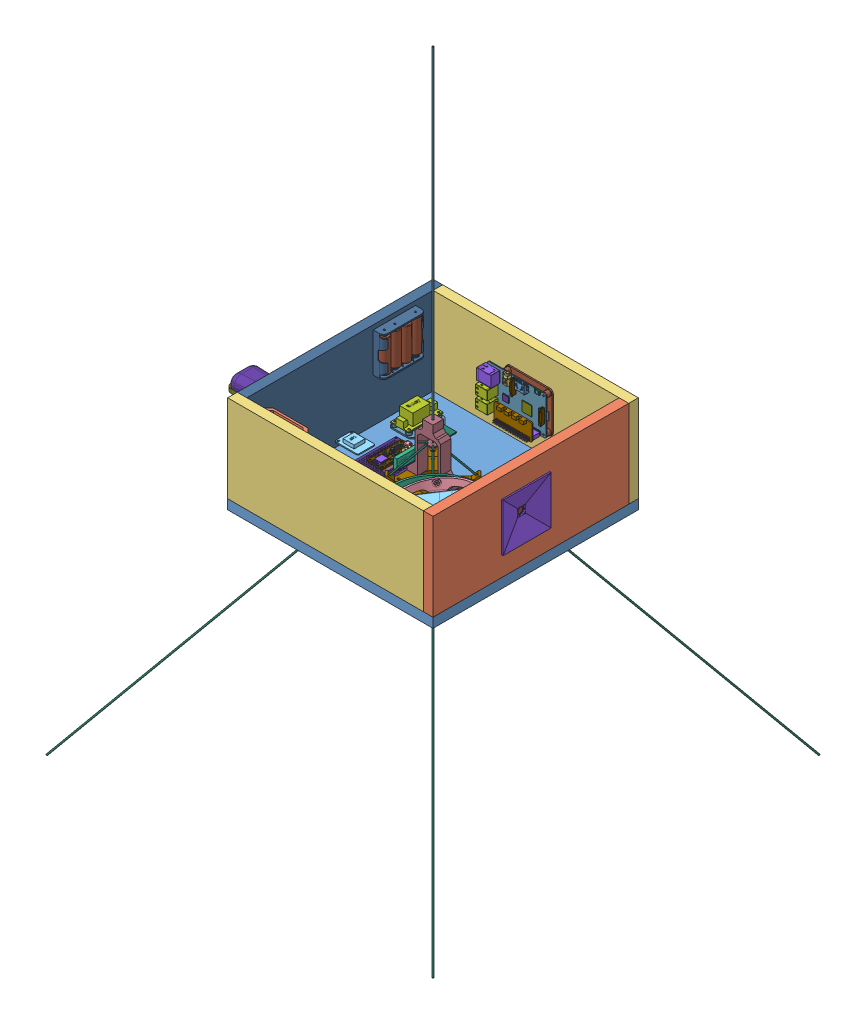
SolidWorks assembly payload_assembly, configuration Default. Lengths in mm.
Overall size (563.71 892.13 563.71).
118 component instances, 78 part files, 109 mates.
Components (placement in the parent):
- payload_bottom-1: payload_bottom [Default] at (116.8734 114.9851 255.4701) size (298.45 13.97 298.45)
- payload_left-1: payload_left [Default] at (266.0984 192.4551 262.4551) x (0 0 1) z (0 -1 0) size (284.48 13.97 127)
- payload_back-1: payload_back [Default] at (123.8584 192.4551 120.2151) x (1 0 0) z (0 1 0) size (284.48 13.97 127)
- gyro-1: gyro [Default] at (171.8134 133.4585 242.8239) x (0.984477 0.175396 -0.006382) z (0.009 -0.014135 0.99986) size (168.98 93.78 168.98) (flexible)
  - gyro_inner-1: gyro_inner [Default] at (30.4784 52.5911 82.2076) size (101.6 33.56 101.6)
  - SPOT3-1: SPOT3 [Default] at (31.7052 32.5911 82.7192) x (0.707107 0 -0.707107) z (0.707107 0 0.707107) size (87.12 25.65 65.02)
  - gyro_middle-1: gyro_middle [Default] at (30.5917 52.6347 83.2295) x (0.700643 -0.134899 -0.700643) z (0.095388 0.990859 -0.095388) size (119.38 119.38 9.62)
  - gyro_outer-1: gyro_outer [Default] at (19.6317 -6.8713 83.6693) x (0.691618 -0.112986 0.713372) z (-0.700643 0.134899 0.700643) size (62.5 70 132)
- 40Pin-1: 40Pin [Default] at (148.3591 161.2851 143.0651) x (0 -1 0) z (1 0 0) size (5 18.05 51.4)
- qwiik_board-1: qwiik_board [Default] at (122.4891 172.8551 144.8299) x (-1 0 0) z (0 -1 0) size (55 6.08 25)
- Batterie nel portabatterie-1: Batterie nel portabatterie [Default] at (-12.2822 239.5657 176.5362) x (0 -1 0) z (1 0 0) size (59.56 61.47 15.11)
  - User Library-R6_AA_UM3-1_5V_holder4AA-2: User Library-R6_AA_UM3-1_5V_holder4AA [4AA] at (18.4086 0.1871 -6.0993) size (59.56 61.47 15.11)
  - Batteria ricaricabile stilo-8: Batteria ricaricabile stilo [Default] at (-4.4514 -22.4504 1.9152) x (0 0 -1) z (1 0 0) size (13.97 13.97 50.04)
  - Batteria ricaricabile stilo-9: Batteria ricaricabile stilo [Default] at (41.2686 -7.3064 2.0287) x (0 0 1) z (-1 0 0) size (13.97 13.97 50.04)
  - Batteria ricaricabile stilo-10: Batteria ricaricabile stilo [Default] at (-4.4514 7.7591 1.9152) x (0 0 -1) z (1 0 0) size (13.97 13.97 50.04)
  - Batteria ricaricabile stilo-11: Batteria ricaricabile stilo [Default] at (-7.4994 22.8246 1.9152) x (0 0 -1) z (1 0 0) size (13.97 13.97 50.04)
- bno055_imu-1: bno055_imu [Default] at (116.8734 136.9851 296.0901) x (-1 0 0) z (0 0 -1) size (26.67 5.7 20.32)
- quarter_wave_antenna-1: quarter_wave_antenna [Default] at (124.936 209.8086 253.2076) x (0 0 1) z (0 -1 0) size (563.71 563.71 892.13)
  - sma_panel_mount-1: sma_panel_mount [Default] at (2.2625 8.0626 10.4072) size (12.7 12.7 14.61)
  - quarter_wave_monopole-1: quarter_wave_monopole [Default] at (2.2625 8.0626 -488.1928) x (1 0 0) z (0 -1 0) size (2 493.5 2)
  - quarter_wave_radial-1: quarter_wave_radial [Default] at (6.5625 12.3626 12.4072) x (0.707107 0.707107 0) z (0 0 1) size (392.53 2 395.53)
  - quarter_wave_radial-2: quarter_wave_radial [Default] at (6.5625 3.7626 12.4072) x (0.707107 -0.707107 0) z (0 0 1) size (392.53 2 395.53)
  - quarter_wave_radial-3: quarter_wave_radial [Default] at (-2.0375 3.7626 12.4072) x (-0.707107 -0.707107 0) z (0 0 1) size (392.53 2 395.53)
  - quarter_wave_radial-4: quarter_wave_radial [Default] at (-2.0375 12.3626 12.4072) x (-0.707107 0.707107 0) z (0 0 1) size (392.53 2 395.53)
- mpl3115a2_altimeter-1: mpl3115a2_altimeter [Default] at (207.6784 186.1051 99.8951) x (-1 0 0) z (0 0 -1) size (19.05 17.78 2.6)
- protoboard_assembly-1: protoboard_assembly [Default] at (15.0551 85.9872 207.5123) x (0 0 1) z (0 1 0) size (70 82.89 26.5)
  - protoboard-1: protoboard [Default] at (39.9767 30.2093 49.9679) size (70 50 1.55)
  - feather_sense-1: feather_sense [Default] at (11.5967 19.6493 56.4679) size (51.35 22.86 6.79)
    - feather_sense.step-1: feather_sense.step [Default] at origin size (51.35 22.86 6.79)
      - PCB Component.step-1: PCB Component.step [Default] at origin size (51.35 22.86 6.79)
        - Board.step-1: Board.step [Default] at origin size (50.8 22.86 1.99)
        - KMR2.step-1: KMR2.step [Default] at (11.1 6.223 1.99) size (4.6 2.8 1.94)
        - KMR2.step-2: KMR2.step [Default] at (29.934 5.855 1.99) size (4.6 2.8 1.94)
        - AP2112(3.3V).step-1: AP2112(3.3V).step [Default] at (15.138 9.144 1.99) x (-1 0 0) z (0 0 1) size (3 3 1.4)
        - AP2112(3.3V).step-2: AP2112(3.3V).step [Default] at (18.783 13.386 1.99) x (-1 0 0) z (0 0 1) size (3 3 1.4)
        - RED.step-1: RED.step [Default] at (2.083 5.639 1.99) x (0 -1 0) z (0 0 1) size (1.25 2.02 1.1)
        - RED.step-2: RED.step [Default] at (2.222 17.272 1.99) x (0 1 0) z (0 0 1) size (1.25 2.02 1.1)
        - 4u20329.step-1: 4u20329.step [Default] at (4.445 11.43 1.99) x (0 -1 0) z (0 0 1) size (8.8 5.6 3)
        - MBR054.step-1: MBR054.step [Default] at (10.262 12.395 1.99) x (-1 0 0) z (0 0 1) size (3.6 1.4 1.35)
        - DMG2305.step-1: DMG2305.step [Default] at (9.817 9.55 1.99) size (3.04 2.64 1.12)
        - BLUE.step-1: BLUE.step [Default] at (45.339 18.034 1.99) x (-1 0 0) z (0 0 1) size (0.79 1.6 0.71)
        - MDBT50.step-1: MDBT50.step [Default] at (42.545 11.43 1.99) x (0 -1 0) z (0 0 1) size (10.5 15.5 2.05)
        - GD25Q16.step-1: GD25Q16.step [Default] at (40.767 4.953 1.99) x (-1 0 0) z (0 0 1) size (3 2 0.8)
        - WS2812B3535.step-1: WS2812B3535.step [Default] at (19.387 6.145 1.99) x (-1 0 0) z (0 0 1) size (3.5 3.5 1.2)
        - 2.2K.step-1: 2.2K.step [Default] at (19.075 8.788 1.99) size (1.6 0.9 0.8)
        - 2.2K.step-2: 2.2K.step [Default] at (31.306 10.198 1.99) size (1.6 0.9 0.8)
        - 2.2K.step-3: 2.2K.step [Default] at (6.756 7.379 1.99) x (0 1 0) z (0 0 1) size (1.6 0.9 0.8)
        - 2.2K.step-4: 2.2K.step [Default] at (15.316 5.309 1.99) size (1.6 0.9 0.8)
        - 2.2K.step-5: 2.2K.step [Default] at (35.878 5.398 1.99) size (1.6 0.9 0.8)
        - 2.2K.step-6: 2.2K.step [Default] at (36.83 4.128 1.99) size (1.6 0.9 0.8)
        - 2.2K.step-7: 2.2K.step [Default] at (33.274 16.637 1.99) x (0 1 0) z (0 0 1) size (1.6 0.9 0.8)
        - 2.2K.step-8: 2.2K.step [Default] at (26.162 17.208 1.99) x (0 -1 0) z (0 0 1) size (1.6 0.9 0.8)
        - 2.2K.step-9: 2.2K.step [Default] at (31.306 11.494 1.99) size (1.6 0.9 0.8)
        - 2.2K.step-10: 2.2K.step [Default] at (24.828 17.208 1.99) x (0 -1 0) z (0 0 1) size (1.6 0.9 0.8)
        - 2.2K.step-11: 2.2K.step [Default] at (5.715 19.685 1.99) x (0 -1 0) z (0 0 1) size (1.6 0.9 0.8)
        - 10uF.step-1: 10uF.step [Default] at (18.796 10.376 1.99) size (2 1.25 1)
        - 10uF.step-2: 10uF.step [Default] at (21.082 17.907 1.99) x (-1 0 0) z (0 0 1) size (2 1.25 1)
        - 10uF.step-3: 10uF.step [Default] at (12.294 9.855 1.99) x (0 1 0) z (0 0 1) size (2 1.25 1)
        - 10uF.step-4: 10uF.step [Default] at (31.306 8.712 1.99) size (2 1.25 1)
        - 10uF.step-5: 10uF.step [Default] at (15.316 12.256 1.99) x (-1 0 0) z (0 0 1) size (2 1.25 1)
        - DNP.step-1: DNP.step [Default] at (33.82 9.373 1.99) x (0 -1 0) z (0 0 1) size (2 1.25 0.85)
        - 4.7K.step-1: 4.7K.step [Default] at (17.374 17.501 1.99) x (-1 0 0) z (0 0 1) size (3.05 1.6 0.5)
        - 4.7K.step-2: 4.7K.step [Default] at (42.608 18.224 1.99) x (-1 0 0) z (0 0 1) size (3.05 1.6 0.5)
        - LSM6DS33.step-1: LSM6DS33.step [Default] at (22.416 14.542 1.99) x (0 1 0) z (0 0 1) size (3 3 1)
        - LIS3MDL.step-1: LIS3MDL.step [Default] at (25.844 13.398 1.99) x (-1 0 0) z (0 0 1) size (2 2 0.7)
        - APDS-9960.step-1: APDS-9960.step [Default] at (26.352 10.224 1.99) x (0 1 0) z (0 0 1) size (2.36 3.94 1.36)
        - SHT30.step-1: SHT30.step [Default] at (22.479 10.668 1.99) size (2.4 2.4 1)
        - MIC_PDM.step-1: MIC_PDM.step [Default] at (30.544 17.272 1.99) x (0 1 0) z (0 0 1) size (3 4 1.06)
        - BMP280.step-1: BMP280.step [Default] at (23.241 6.985 1.99) x (-1 0 0) z (0 0 1) size (2 2.5 0.97)
        - CON_JST_PH_2PIN_MTPH2.step-1: CON_JST_PH_2PIN_MTPH2.step [Default] at (10.795 19.304 1.99) size (7.9 8.6 4.8)
  - 12pin-header-1: 12pin-header [Default] at (42.9767 41.2593 56.4679) x (1 0 0) z (0 1 0) size (30.98 8 2.5)
  - 12pin-header-2: 12pin-header [Default] at (42.9767 20.8993 56.4679) x (1 0 0) z (0 1 0) size (30.98 8 2.5)
  - ultimate_gps-1: ultimate_gps [Default] at (49.6967 -10.0687 56.9579) x (0 -1 0) z (-1 0 0) size (34.04 6.5 25.4)
  - hx1_radio-1: hx1_radio [Default] at (32.8267 50.7993 65.7079) x (-1 0 0) z (0 0 -1) size (43 5 26.5)
- relay-1: relay [Default] at (9.5684 134.9551 171.6151) x (0 0 -1) z (1 0 0) size (50.04 18.52 25.91)
- arducam_usb_holder-1: arducam_usb_holder [Default] at (255.0984 192.4551 269.9227) x (0 -1 0) z (0 0 1) size (70 13 70)
- arducam_csi_holder-1: arducam_csi_holder [Default] at (116.8734 108.9851 255.4701) x (-1 0 0) z (0 0 -1) size (88.89 15 74)
- arducam_csi-2: arducam_csi [Default] at (116.8734 125.4851 255.4701) x (0 0 -1) z (-1 0 0) size (36 37.5 36)
- arducam_usb-2: arducam_usb [Default] at (253.5984 192.4551 270.5877) x (0 0 -1) z (0 -1 0) size (31 4.5 31)
- mpl3115a2_altimeter_holder-1: mpl3115a2_altimeter_holder [Default] at (198.1534 198.8051 106.2451) x (-1 0 0) z (0 -1 0) size (31.75 6.35 38.1)
- mpl3115a2_altimeter_cover-1: mpl3115a2_altimeter_cover [Default] at (198.1534 198.8051 90.3701) x (1 0 0) z (0 -1 0) size (31.75 12.7 38.1)
- payload_top-1: payload_top [Default] at (266.0984 114.9851 -29.0099) size (298.45 13.97 298.45) (hidden)
- RaspberryPi2-1: RaspberryPi2 [Default] at (112.4891 188.3551 129.5151) x (-1 0 0) z (0 1 0) size (89.62 18.75 58.3)
  - RaspberryPi2 STEP214.STEP-1: RaspberryPi2 STEP214.STEP [Default] at origin size (89.62 18.75 58.3)
    - Mainboard2.STEP-1: Mainboard2.STEP [Default] at origin size (85 1.3 56)
    - GPIO.STEP-1: GPIO.STEP [Default] at (-11.37 0 -24.5) x (0 0 1) z (-1 0 0) size (5 11.5 50.8)
    - Processor.STEP-1: Processor.STEP [Default] at (-15.5 0 -3) x (0 0 1) z (-1 0 0) size (14 1 14)
    - GPU.STEP-1: GPU.STEP [Default] at (15.25 0 -5.75) x (0 0 1) z (-1 0 0) size (9.1 1 9.1)
    - CameraAssembly.STEP-1: CameraAssembly.STEP [Default] at (10.0885 -2.9159 16.55) x (-1 0 0) z (0 0 -1) size (5.01 5.51 22.11)
    - CameraAssembly.STEP-2: CameraAssembly.STEP [Default] at (-46.3885 -2.9159 0) size (5.01 5.51 22.11)
    - HDMI.STEP-1: HDMI.STEP [Default] at (-10.2 0.27 29.3) size (15.04 8.38 12.15)
    - RAM.STEP-1: RAM.STEP [Default] at (0.5 -2.3 -6) x (0 0 1) z (-1 0 0) size (12 1 12)
    - Audio.STEP-1: Audio.STEP [Default] at (10.9 0.15 21.75) size (7 6 14.8)
    - MicroSDSocket.STEP-1: MicroSDSocket.STEP [Default] at (-34.5 -1.3 -0.7) x (0 0 -1) z (-1 0 0) size (13 1.3 14)
    - MicroSD.STEP-1: MicroSD.STEP [Default] at (-37 -2.3 0.1) x (0 0 1) z (-1 0 0) size (11.01 1 15)
    - micro USB2.STEP-1: micro USB2.STEP [Default] at (-17.2704 -5.0969 44.9026) size (7.98 2.93 5.58)
    - usb double.STEP-1: usb double.STEP [Default] at (30.38 -0.09 -18.85) x (0 0 -1) z (1 0 0) size (15.6 18.75 17.92)
    - usb double.STEP-2: usb double.STEP [Default] at (30.38 -0.09 -1.25) x (0 0 -1) z (1 0 0) size (15.6 18.75 17.92)
    - RJ45-LED.STEP-1: RJ45-LED.STEP [Default] at (34.11 7.4 17.348) x (1 0 0) z (0 -1 0) size (21.3 18 14.1)
- antenna_holder_middle-1: antenna_holder_middle [Default] at (116.8734 123.9851 255.4701) x (-1 0 0) z (0 0 -1) size (77.07 37.17 77.07)
- payload_right-2: payload_right [Default] at (-32.3516 192.4551 248.4851) x (0 0 -1) z (0 -1 0) size (284.48 13.97 127)
- payload_back-2: payload_back [Default] at (109.8884 192.4551 404.6951) x (-1 0 0) z (0 -1 0) size (284.48 13.97 127)
- pi_holder-1: pi_holder [Default] at (122.4891 188.3551 120.2151) size (68 59 8)
- antenna_bracer-1: antenna_bracer [Default] at (41.7963 97.3074 180.3929) x (-0.5 0.707107 -0.5) z (0.707107 0 -0.707107) size (20 52.17 20)
- antenna_bracer-2: antenna_bracer [Default] at (41.7963 97.3074 330.5473) x (-0.5 0.707107 0.5) z (-0.707107 0 -0.707107) size (20 52.17 20)
- antenna_bracer-3: antenna_bracer [Default] at (191.9506 97.3074 330.5473) x (0.5 0.707107 0.5) z (-0.707107 0 0.707107) size (20 52.17 20)
- antenna_bracer-4: antenna_bracer [Default] at (191.9506 97.3074 180.3929) x (0.5 0.707107 -0.5) z (0.707107 0 0.707107) size (20 52.17 20)
- antenna_holder_top-1: antenna_holder_top [Default] at (116.8734 153.9851 255.4701) size (60 75 15)
- power_system_holder-1: power_system_holder [Default] at (14.3184 128.9551 171.6151) x (0 0 1) z (-1 0 0) size (52 6 40)
- power_board-1: power_board [Default] at (42.3184 134.9551 171.6151) x (-1 0 0) z (0 0 -1) size (30 1.5 20)
- gps_antenna_holder-1: gps_antenna_holder [Default] at (-32.3516 225.9551 360.7251) x (0 -1 0) z (1 0 0) size (34.5 38 46)
- gps_antenna-1: gps_antenna [Default] at (-53.6353 225.9551 341.6893) size (50 15.5 38.09)
- icm20984_imu_holder-1: icm20984_imu_holder [Default] at (116.8734 136.9851 321.7101) x (-1 0 0) z (0 0 1) size (30 7 60)
- icm20984_imu-1: icm20984_imu [Default] at (116.8734 136.9851 321.7101) size (26 4.6 26)
- hot_hand_holder-1: hot_hand_holder [Default] at (26.0684 186.1051 371.6751) x (0 -1 0) z (-1 0 0) size (114.3 19.05 63.5)
- protoboard_holder-1: protoboard_holder [Default] at (45.2644 128.9551 246.489) x (0 0 1) z (-1 0 0) size (72.35 7 52)
- pi_zero_holder-1: pi_zero_holder [Default] at (252.1284 209.2551 210.7227) x (0 1 0) z (-1 0 0) size (68 33 8)
- RaspberryPiZeroW-1: RaspberryPiZeroW [Default] at (244.1284 209.0582 211.2915) x (0 0.999823 0.018804) z (0 -0.018804 0.999823) size (65.9 4.8 31.25)
Mates (geometry in assembly coordinates):
- Coincident10: coincident anti-aligned: plane of payload_left-1 through (252.1284 128.9551 120.2151) normal (0 0 -1); plane of payload_back-1 through (123.8584 192.4551 120.2151) normal (0 0 1)
- Parallel3: parallel anti-aligned: plane of payload_back-1 through (123.8584 192.4551 106.2451) normal (0 0 -1); plane of quarter_wave_antenna-1/sma_panel_mount-1 through (121.8372 197.8014 261.8201) normal (0 0 1)
- Coincident56: coincident anti-aligned: plane of payload_left-1 through (266.0984 162.4551 239.9227) normal (0 1 0); plane of arducam_usb_holder-1 through (261.0984 162.4551 299.9227) normal (0 -1 0)
- Coincident57: coincident anti-aligned: plane of payload_left-1 through (266.0984 192.4551 262.4551) normal (1 0 0); plane of arducam_usb_holder-1 through (266.0984 192.4551 269.9227) normal (-1 0 0)
- Coincident58: coincident anti-aligned: plane of payload_left-1 through (266.0984 162.4551 299.9227) normal (0 0 -1); plane of arducam_usb_holder-1 through (261.0984 222.4551 299.9227) normal (0 0 1)
- Coincident61: coincident anti-aligned: plane of payload_bottom-1 through (116.8734 114.9851 255.4701) normal (0 -1 0); plane of arducam_csi_holder-1 through (116.8734 114.9851 255.4701) normal (0 1 0)
- Concentric3: concentric anti-aligned: cylinder of arducam_csi_holder-1 through (102.8734 117.9851 241.4701) axis (0 1 0) radius 1.5; cylinder of arducam_csi-2 through (102.8734 125.4851 241.4701) axis (0 -1 0) radius 1.5
- Coincident63: coincident anti-aligned: plane of arducam_csi_holder-1 through (116.8734 123.9851 255.4701) normal (0 1 0); plane of arducam_csi-2 through (116.8734 123.9851 255.4701) normal (0 -1 0)
- Concentric4: concentric anti-aligned: cylinder of arducam_csi_holder-1 through (130.8734 117.9851 241.4701) axis (0 1 0) radius 1.5; cylinder of arducam_csi-2 through (130.8734 125.4851 241.4701) axis (0 -1 0) radius 1.5
- Concentric5: concentric anti-aligned: cylinder of arducam_usb_holder-1 through (258.0984 206.4551 256.5877) axis (-1 0 0) radius 0.925; cylinder of arducam_usb-2 through (253.5984 206.4551 256.5877) axis (1 0 0) radius 1.25
- Parallel5: parallel aligned: plane of payload_left-1 through (266.0984 162.4551 239.9227) normal (0 1 0); plane of arducam_usb-2 through (255.0984 207.9551 286.0877) normal (0 1 0)
- Coincident65: coincident anti-aligned: plane of arducam_usb_holder-1 through (255.0984 192.4551 269.9227) normal (-1 0 0); plane of arducam_usb-2 through (255.0984 192.4551 270.5877) normal (1 0 0)
- Concentric8: concentric aligned: cylinder of mpl3115a2_altimeter-1 through (205.1384 201.3451 99.8951) axis (0 0 -1) radius 1.27; cylinder of mpl3115a2_altimeter_holder-1 through (205.1384 201.3451 106.2451) axis (0 0 -1) radius 0.875
- Coincident70: coincident anti-aligned: plane of mpl3115a2_altimeter-1 through (198.1534 194.9951 99.8951) normal (0 0 1); plane of mpl3115a2_altimeter_holder-1 through (198.1534 198.8051 99.8951) normal (0 0 -1)
- Parallel7: parallel aligned: plane of mpl3115a2_altimeter-1 through (188.6284 188.6451 99.8951) normal (-1 0 0); plane of mpl3115a2_altimeter_holder-1 through (184.9454 182.4221 103.0701) normal (-1 0 0)
- Concentric11: concentric aligned: cylinder of mpl3115a2_altimeter_holder-1 through (205.1384 211.5051 106.2451) axis (0 0 -1) radius 0.875; cylinder of mpl3115a2_altimeter_cover-1 through (205.1384 211.5051 103.0701) axis (0 0 -1) radius 1.375
- Concentric12: concentric aligned: cylinder of mpl3115a2_altimeter_holder-1 through (191.1684 211.5051 106.2451) axis (0 0 -1) radius 0.875; cylinder of mpl3115a2_altimeter_cover-1 through (191.1684 211.5051 103.0701) axis (0 0 -1) radius 1.375
- Coincident72: coincident anti-aligned: plane of mpl3115a2_altimeter_holder-1 through (198.1534 198.8051 99.8951) normal (0 0 -1); plane of mpl3115a2_altimeter_cover-1 through (198.1534 198.8051 99.8951) normal (0 0 1)
- Coincident73: coincident anti-aligned: plane of payload_back-1 through (-18.3816 128.9551 106.2451) normal (0 -1 0); plane of payload_top-1 through (266.0984 128.9551 -29.0099) normal (0 1 0)
- Coincident75: coincident aligned: plane of payload_back-1 through (123.8584 192.4551 120.2151) normal (0 0 1); plane of payload_top-1 through (116.8734 128.9551 120.2151) normal (0 0 1)
- Coincident78: coincident aligned: plane of 40Pin-1 through (98.2091 165.3751 143.0651) normal (-1 0 0); plane of RaspberryPi2-1/RaspberryPi2 STEP214.STEP-1/GPIO.STEP-1 through (98.2091 165.1251 132.0151) normal (-1 0 0)
- Coincident79: coincident anti-aligned: plane of 40Pin-1 through (122.6591 163.7851 132.0151) normal (0 0 -1); plane of RaspberryPi2-1/RaspberryPi2 STEP214.STEP-1/GPIO.STEP-1 through (123.8591 163.8551 132.0151) normal (0 0 1)
- Coincident80: coincident aligned: plane of 40Pin-1 through (98.8491 165.3751 143.0651) normal (0 1 0); plane of RaspberryPi2-1/RaspberryPi2 STEP214.STEP-1/GPIO.STEP-1 through (98.7091 165.3751 132.0151) normal (0 1 0)
- Coincident81: coincident aligned: plane of payload_left-1 through (266.0984 192.4551 262.4551) normal (1 0 0); plane of payload_back-1 through (266.0984 255.9551 106.2451) normal (1 0 0)
- Coincident86: coincident aligned: plane of qwiik_board-1 through (149.9891 160.3551 143.0651) normal (0 -1 0); plane of RaspberryPi2-1/RaspberryPi2 STEP214.STEP-1/Mainboard2.STEP-1 through (72.4891 160.3551 128.2151) normal (0 -1 0)
- Coincident87: coincident anti-aligned: plane of qwiik_board-1 through (149.9891 160.3551 143.0651) normal (1 0 0); plane of RaspberryPi2-1/RaspberryPi2 STEP214.STEP-1/CameraAssembly.STEP-2 through (149.9891 198.6051 129.5151) normal (-1 0 0)
- Coincident88: coincident anti-aligned: plane of 40Pin-1 through (122.6591 163.7851 143.0651) normal (0 0 1); plane of qwiik_board-1 through (122.4891 172.8551 143.0651) normal (0 0 -1)
- Coincident91: coincident anti-aligned: plane of arducam_csi_holder-1 through (116.8734 123.9851 255.4701) normal (0 1 0); plane of antenna_holder_middle-1 through (116.8734 123.9851 255.4701) normal (0 -1 0)
- Concentric17: concentric anti-aligned: cylinder of RaspberryPi2-1/RaspberryPi2 STEP214.STEP-1/Mainboard2.STEP-1 through (93.4891 212.8551 128.2151) axis (0 0 1) radius 1.25; cylinder of pi_holder-1 through (93.4891 212.8551 122.2151) axis (0 0 -1) radius 0.95
- Concentric18: concentric anti-aligned: cylinder of RaspberryPi2-1/RaspberryPi2 STEP214.STEP-1/Mainboard2.STEP-1 through (151.4891 212.8551 128.2151) axis (0 0 1) radius 1.25; cylinder of pi_holder-1 through (151.4891 212.8551 122.2151) axis (0 0 -1) radius 0.95
- Concentric19: concentric aligned: cylinder of arducam_csi_holder-1 through (141.8734 118.9851 280.4701) axis (0 1 0) radius 1.875; cylinder of antenna_holder_middle-1 through (141.8734 123.9851 280.4701) axis (0 1 0) radius 1.875
- Concentric20: concentric aligned: cylinder of arducam_csi_holder-1 through (91.8734 118.9851 280.4701) axis (0 1 0) radius 1.875; cylinder of antenna_holder_middle-1 through (91.8734 123.9851 280.4701) axis (0 1 0) radius 1.875
- Concentric25: concentric aligned: cylinder of quarter_wave_antenna-1/quarter_wave_radial-4 through (112.2628 196.9621 250.8595) axis (-0.5 -0.707107 -0.5) radius 1; cylinder of antenna_bracer-1 through (59.2963 122.0561 197.8929) axis (-0.5 -0.707107 -0.5) radius 1.905
- Concentric26: concentric anti-aligned: cylinder of quarter_wave_antenna-1/quarter_wave_radial-1 through (112.2628 196.9621 260.0808) axis (-0.5 -0.707107 0.5) radius 1; cylinder of antenna_holder_middle-1 through (69.4991 136.4851 302.8445) axis (0.5 0.707107 -0.5) radius 1.5
- Concentric27: concentric anti-aligned: cylinder of quarter_wave_antenna-1/quarter_wave_radial-4 through (112.2628 196.9621 250.8595) axis (-0.5 -0.707107 -0.5) radius 1; cylinder of antenna_holder_middle-1 through (69.4991 136.4851 208.0957) axis (0.5 0.707107 0.5) radius 1.5
- Coincident109: coincident anti-aligned: plane of payload_bottom-1 through (116.8734 114.9851 255.4701) normal (0 -1 0); plane of antenna_bracer-1 through (17.2252 114.9851 209.964) normal (0 1 0)
- Concentric28: concentric aligned: cylinder of quarter_wave_antenna-1/quarter_wave_radial-1 through (112.2628 196.9621 260.0808) axis (-0.5 -0.707107 0.5) radius 1; cylinder of antenna_bracer-2 through (59.2963 122.0561 313.0473) axis (-0.5 -0.707107 0.5) radius 1.905
- Coincident110: coincident anti-aligned: plane of payload_bottom-1 through (116.8734 114.9851 255.4701) normal (0 -1 0); plane of antenna_bracer-2 through (71.3674 114.9851 355.1183) normal (0 1 0)
- Coincident111: coincident anti-aligned: plane of payload_bottom-1 through (116.8734 114.9851 255.4701) normal (0 -1 0); plane of antenna_bracer-3 through (216.5217 114.9851 300.9762) normal (0 1 0)
- Concentric29: concentric aligned: cylinder of quarter_wave_antenna-1/quarter_wave_radial-2 through (121.4841 196.9621 260.0808) axis (0.5 -0.707107 0.5) radius 1; cylinder of antenna_bracer-3 through (174.4506 122.0561 313.0473) axis (0.5 -0.707107 0.5) radius 1.905
- Concentric30: concentric aligned: cylinder of quarter_wave_antenna-1/quarter_wave_radial-3 through (121.4841 196.9621 250.8595) axis (0.5 -0.707107 -0.5) radius 1; cylinder of antenna_bracer-4 through (174.4506 122.0561 197.8929) axis (0.5 -0.707107 -0.5) radius 1.905
- Coincident112: coincident anti-aligned: plane of payload_bottom-1 through (116.8734 114.9851 255.4701) normal (0 -1 0); plane of antenna_bracer-4 through (162.3795 114.9851 155.8219) normal (0 1 0)
- Concentric31: concentric anti-aligned: cylinder of antenna_holder_middle-1 through (94.3734 123.9851 255.4701) axis (0 1 0) radius 1.875; cylinder of antenna_holder_top-1 through (94.3734 158.9851 255.4701) axis (0 -1 0) radius 1.875
- Concentric32: concentric anti-aligned: cylinder of antenna_holder_middle-1 through (139.3734 123.9851 255.4701) axis (0 1 0) radius 1.875; cylinder of antenna_holder_top-1 through (139.3734 158.9851 255.4701) axis (0 -1 0) radius 1.875
- Coincident113: coincident anti-aligned: plane of antenna_holder_middle-1 through (116.8734 153.9851 255.4701) normal (0 1 0); plane of antenna_holder_top-1 through (116.8734 153.9851 255.4701) normal (0 -1 0)
- Coincident114: coincident anti-aligned: plane of payload_bottom-1 through (116.8734 128.9551 255.4701) normal (0 1 0); plane of power_system_holder-1 through (14.3184 128.9551 171.6151) normal (0 -1 0)
- Concentric33: concentric anti-aligned: cylinder of relay-1 through (-0.6816 153.4731 150.1151) axis (0 -1 0) radius 1.5; cylinder of power_system_holder-1 through (-0.6816 128.9551 150.1151) axis (0 1 0) radius 1.375
- Concentric34: concentric anti-aligned: cylinder of relay-1 through (19.8184 153.4731 150.1151) axis (0 -1 0) radius 1.5; cylinder of power_system_holder-1 through (19.8184 128.9551 150.1151) axis (0 1 0) radius 1.375
- Coincident116: coincident anti-aligned: plane of relay-1 through (9.5684 134.9551 171.6151) normal (0 -1 0); plane of power_system_holder-1 through (-0.6816 134.9551 193.1151) normal (0 1 0)
- Concentric35: concentric aligned: cylinder of power_system_holder-1 through (29.3184 128.9551 163.6151) axis (0 1 0) radius 0.9; cylinder of power_board-1 through (29.3184 134.9551 163.6151) axis (0 1 0) radius 1.25
- Concentric36: concentric aligned: cylinder of power_system_holder-1 through (29.3184 128.9551 179.6151) axis (0 1 0) radius 0.9; cylinder of power_board-1 through (29.3184 134.9551 179.6151) axis (0 1 0) radius 1.25
- Coincident118: coincident anti-aligned: plane of power_system_holder-1 through (29.3184 134.9551 179.6151) normal (0 1 0); plane of power_board-1 through (42.3184 134.9551 171.6151) normal (0 -1 0)
- Coincident119: coincident anti-aligned: plane of payload_right-2 through (-32.3516 192.4551 248.4851) normal (-1 0 0); plane of gps_antenna_holder-1 through (-32.3516 191.4551 322.7251) normal (1 0 0)
- Distance30: distance = 30 mm aligned: plane of gps_antenna_holder-1 through (-32.3516 225.9551 322.7251) normal (0 1 0); plane of payload_right-2 through (-18.3816 255.9551 390.7251) normal (0 1 0)
- Distance31: distance = 30 mm aligned: plane of gps_antenna_holder-1 through (-32.3516 225.9551 360.7251) normal (0 0 1); plane of payload_right-2 through (-18.3816 128.9551 390.7251) normal (0 0 1)
- Coincident122: coincident anti-aligned: plane of gps_antenna_holder-1 through (-32.3516 225.9551 322.7251) normal (0 1 0); plane of gps_antenna-1 through (-53.6353 225.9551 341.6893) normal (0 -1 0)
- Coincident123: coincident anti-aligned: plane of payload_right-2 through (-32.3516 192.4551 248.4851) normal (-1 0 0); plane of gps_antenna-1 through (-32.3516 241.4551 359.1893) normal (1 0 0)
- Coincident124: coincident: line of gps_antenna_holder-1 through (-71.3516 225.9551 360.7251) axis (1 0 0); point of gps_antenna-1
- Coincident139: coincident anti-aligned: plane of payload_bottom-1 through (86.8734 114.9851 285.4701) normal (0 0 -1); plane of arducam_csi_holder-1 through (146.8734 123.9851 285.4701) normal (0 0 1)
- Coincident140: coincident anti-aligned: plane of payload_bottom-1 through (146.8734 114.9851 285.4701) normal (-1 0 0); plane of arducam_csi_holder-1 through (146.8734 123.9851 225.4701) normal (1 0 0)
- Coincident143: coincident aligned: plane of payload_bottom-1 through (266.0984 128.9551 404.6951) normal (1 0 0); plane of payload_left-1 through (266.0984 192.4551 262.4551) normal (1 0 0)
- Coincident144: coincident anti-aligned: plane of payload_bottom-1 through (116.8734 128.9551 255.4701) normal (0 1 0); plane of payload_left-1 through (252.1284 128.9551 120.2151) normal (0 -1 0)
- Coincident146: coincident aligned: plane of payload_bottom-1 through (-32.3516 128.9551 404.6951) normal (0 0 1); plane of payload_left-1 through (252.1284 128.9551 404.6951) normal (0 0 1)
- Coincident147: coincident aligned: plane of payload_left-1 through (252.1284 255.9551 120.2151) normal (0 1 0); plane of payload_back-1 through (-18.3816 255.9551 106.2451) normal (0 1 0)
- Coincident149: coincident anti-aligned: plane of payload_bottom-1 through (116.8734 128.9551 255.4701) normal (0 1 0); plane of payload_right-2 through (-18.3816 128.9551 390.7251) normal (0 -1 0)
- Coincident150: coincident aligned: plane of payload_bottom-1 through (-32.3516 128.9551 404.6951) normal (-1 0 0); plane of payload_right-2 through (-32.3516 192.4551 248.4851) normal (-1 0 0)
- Coincident151: coincident aligned: plane of payload_back-1 through (123.8584 192.4551 106.2451) normal (0 0 -1); plane of payload_right-2 through (-18.3816 128.9551 106.2451) normal (0 0 -1)
- Coincident152: coincident anti-aligned: plane of payload_bottom-1 through (116.8734 128.9551 255.4701) normal (0 1 0); plane of payload_back-2 through (252.1284 128.9551 390.7251) normal (0 -1 0)
- Coincident154: coincident aligned: plane of payload_right-2 through (-32.3516 192.4551 248.4851) normal (-1 0 0); plane of payload_back-2 through (-32.3516 128.9551 390.7251) normal (-1 0 0)
- Coincident155: coincident aligned: plane of payload_bottom-1 through (-32.3516 128.9551 404.6951) normal (0 0 1); plane of payload_back-2 through (109.8884 192.4551 404.6951) normal (0 0 1)
- Concentric37: concentric aligned: cylinder of antenna_holder_middle-1 through (106.0784 123.9851 280.4701) axis (0 1 0) radius 0.9; cylinder of icm20984_imu_holder-1 through (106.0784 129.9851 280.4701) axis (0 1 0) radius 0.9
- Concentric38: concentric aligned: cylinder of antenna_holder_middle-1 through (127.6684 123.9851 280.4701) axis (0 1 0) radius 0.9; cylinder of icm20984_imu_holder-1 through (127.6684 129.9851 280.4701) axis (0 1 0) radius 0.9
- Coincident156: coincident anti-aligned: plane of antenna_holder_middle-1 through (106.0784 133.9851 280.4701) normal (0 1 0); plane of icm20984_imu_holder-1 through (116.8734 133.9851 321.7101) normal (0 -1 0)
- Concentric39: concentric aligned: cylinder of bno055_imu-1 through (106.0784 136.9851 288.4701) axis (0 1 0) radius 1.27; cylinder of icm20984_imu_holder-1 through (106.0784 129.9851 288.4701) axis (0 1 0) radius 0.9
- Concentric40: concentric aligned: cylinder of bno055_imu-1 through (127.6684 136.9851 303.7101) axis (0 1 0) radius 1.27; cylinder of icm20984_imu_holder-1 through (127.6684 129.9851 303.7101) axis (0 1 0) radius 0.9
- Concentric41: concentric aligned: cylinder of icm20984_imu_holder-1 through (126.8734 129.9851 311.7101) axis (0 1 0) radius 1.4; cylinder of icm20984_imu-1 through (126.8734 136.9851 311.7101) axis (0 1 0) radius 1.625
- Concentric42: concentric aligned: cylinder of icm20984_imu_holder-1 through (106.8734 129.9851 331.7101) axis (0 1 0) radius 1.4; cylinder of icm20984_imu-1 through (106.8734 136.9851 331.7101) axis (0 1 0) radius 1.625
- Coincident157: coincident anti-aligned: plane of icm20984_imu_holder-1 through (116.8734 136.9851 321.7101) normal (0 1 0); plane of icm20984_imu-1 through (116.8734 136.9851 321.7101) normal (0 -1 0)
- Coincident158: coincident anti-aligned: plane of bno055_imu-1 through (116.8734 136.9851 296.0901) normal (0 -1 0); plane of icm20984_imu_holder-1 through (116.8734 136.9851 321.7101) normal (0 1 0)
- Coincident159: coincident anti-aligned: plane of RaspberryPi2-1/RaspberryPi2 STEP214.STEP-1/Mainboard2.STEP-1 through (72.4891 213.8551 128.2151) normal (0 0 -1); plane of pi_holder-1 through (151.4891 212.8551 128.2151) normal (0 0 1)
- Coincident164: coincident anti-aligned: plane of payload_bottom-1 through (116.8734 128.9551 255.4701) normal (0 1 0); plane of power_system_holder-1 through (14.3184 128.9551 171.6151) normal (0 -1 0)
- Distance37: distance = 12.7 mm anti-aligned: plane of power_system_holder-1 through (-5.6816 130.9551 145.6151) normal (-1 0 0); plane of payload_right-2 through (-18.3816 192.4551 248.4851) normal (1 0 0)
- Distance38: distance = 25.4 mm anti-aligned: plane of power_system_holder-1 through (-5.6816 130.9551 145.6151) normal (0 0 -1); plane of payload_back-1 through (123.8584 192.4551 120.2151) normal (0 0 1)
- Concentric43: concentric anti-aligned: cylinder of protoboard_assembly-1/protoboard-1 through (22.2644 136.7051 214.489) axis (0 1 0) radius 1; cylinder of protoboard_holder-1 through (22.2644 131.9551 214.489) axis (0 -1 0) radius 0.875
- Parallel11: parallel aligned: plane of protoboard_assembly-1/protoboard-1 through (70.2644 135.9551 282.489) normal (0 0 1); plane of protoboard_holder-1 through (19.2644 131.9551 282.6629) normal (0 0 1)
- Coincident168: coincident anti-aligned: plane of protoboard_assembly-1/protoboard-1 through (45.2644 135.9551 247.489) normal (0 -1 0); plane of protoboard_holder-1 through (68.2644 135.9551 214.489) normal (0 1 0)
- Distance39: distance = 6.35 mm anti-aligned: plane of protoboard_assembly-1/ultimate_gps-1 through (-12.0316 144.4451 244.509) normal (-1 0 0); plane of payload_right-2 through (-18.3816 192.4551 248.4851) normal (1 0 0)
- Distance40: distance = 12.7 mm anti-aligned: plane of protoboard_holder-1 through (19.2644 131.9551 210.3151) normal (0 0 -1); plane of power_system_holder-1 through (-5.6816 130.9551 197.6151) normal (0 0 1)
- Coincident171: coincident anti-aligned: plane of payload_bottom-1 through (116.8734 128.9551 255.4701) normal (0 1 0); plane of protoboard_holder-1 through (45.2644 128.9551 246.489) normal (0 -1 0)
- Coincident173: coincident anti-aligned: plane of payload_back-2 through (109.8884 192.4551 390.7251) normal (0 0 -1); plane of hot_hand_holder-1 through (26.0684 186.1051 390.7251) normal (0 0 1)
- Distance41: distance = 12.7 mm anti-aligned: plane of hot_hand_holder-1 through (-5.6816 233.7301 371.6751) normal (-1 0 0); plane of payload_right-2 through (-18.3816 192.4551 248.4851) normal (1 0 0)
- Coincident175: coincident anti-aligned: plane of payload_bottom-1 through (116.8734 128.9551 255.4701) normal (0 1 0); plane of hot_hand_holder-1 through (21.3059 128.9551 374.8501) normal (0 -1 0)
- Coincident176: coincident anti-aligned: plane of payload_left-1 through (252.1284 192.4551 262.4551) normal (-1 0 0); plane of pi_zero_holder-1 through (252.1284 209.2551 210.7227) normal (1 0 0)
- Distance42: distance = 12.7 mm aligned: plane of pi_zero_holder-1 through (250.1284 243.2551 227.2227) normal (0 1 0); plane of payload_left-1 through (252.1284 255.9551 120.2151) normal (0 1 0)
- Distance43: distance = 12.7 mm aligned: plane of pi_zero_holder-1 through (250.1284 175.2551 227.2227) normal (0 0 1); plane of payload_left-1 through (266.0984 162.4551 239.9227) normal (0 0 1)
- Concentric45: concentric anti-aligned: cylinder of RaspberryPiZeroW-1 through (244.1284 180.2551 199.2227) axis (-1 0 0) radius 1.325; cylinder of pi_zero_holder-1 through (250.1284 180.2551 199.2227) axis (1 0 0) radius 0.95
- Parallel13: parallel anti-aligned: cylinder of pi_zero_holder-1 through (250.1284 238.2551 222.2227) axis (1 0 0) radius 0.95; cylinder of RaspberryPiZeroW-1 through (244.1284 237.8614 223.3602) axis (-1 0 0) radius 1.325
- Coincident179: coincident anti-aligned: plane of pi_zero_holder-1 through (244.1284 238.2551 199.2227) normal (-1 0 0); plane of RaspberryPiZeroW-1 through (244.1284 180.5248 199.5028) normal (1 0 0)
- Coincident180: coincident anti-aligned: plane of payload_bottom-1 through (116.8734 128.9551 255.4701) normal (0 1 0); plane of gyro-1/gyro_outer-1 through (193.0978 128.9551 326.2497) normal (0 -1 0)
- Distance44: distance = 44.45 mm anti-aligned: plane of gyro-1/gyro_outer-1 through (139.3577 131.9551 365.8477) normal (-0.707107 0 -0.707107); plane of antenna_holder_middle-1 through (148.3379 148.9851 294.0056) normal (0.707107 0 0.707107)
- Distance45: distance = 57.15 mm aligned: plane of gyro-1/gyro_outer-1 through (139.3577 131.9551 365.8477) normal (-0.707107 0 0.707107); plane of antenna_holder_middle-1 through (148.3379 148.9851 294.0056) normal (-0.707107 0 0.707107)
- Coincident184: coincident anti-aligned: plane of Batterie nel portabatterie-1/User Library-R6_AA_UM3-1_5V_holder4AA-2 through (-18.3816 249.6051 207.0831) normal (-1 0 0); plane of payload_right-2 through (-18.3816 192.4551 248.4851) normal (1 0 0)
- Distance46: distance = 6.35 mm aligned: plane of Batterie nel portabatterie-1/User Library-R6_AA_UM3-1_5V_holder4AA-2 through (-3.2686 249.6051 145.6151) normal (0 1 0); plane of payload_right-2 through (-18.3816 255.9551 390.7251) normal (0 1 0)
- Distance47: distance = 25.4 mm anti-aligned: plane of Batterie nel portabatterie-1/User Library-R6_AA_UM3-1_5V_holder4AA-2 through (-3.2686 249.6051 145.6151) normal (0 0 -1); plane of payload_back-1 through (123.8584 192.4551 120.2151) normal (0 0 1)
- Coincident189: coincident anti-aligned: plane of payload_back-1 through (123.8584 192.4551 106.2451) normal (0 0 -1); plane of mpl3115a2_altimeter_holder-1 through (198.1534 198.8051 106.2451) normal (0 0 1)
- Coincident191: coincident aligned: plane of mpl3115a2_altimeter_holder-1 through (214.0284 217.8551 99.8951) normal (0 1 0); plane of pi_holder-1 through (88.4891 217.8551 122.2151) normal (0 1 0)
- Coincident192: coincident anti-aligned: plane of payload_back-1 through (123.8584 192.4551 120.2151) normal (0 0 1); plane of pi_holder-1 through (122.4891 188.3551 120.2151) normal (0 0 -1)
- Distance48: distance = 38.1 mm anti-aligned: plane of mpl3115a2_altimeter_cover-1 through (214.0284 179.7551 93.5451) normal (1 0 0); plane of payload_left-1 through (252.1284 192.4551 262.4551) normal (-1 0 0)
- Distance49: distance = 38.1 mm aligned: plane of mpl3115a2_altimeter_holder-1 through (214.0284 217.8551 99.8951) normal (0 1 0); plane of payload_back-1 through (-18.3816 255.9551 106.2451) normal (0 1 0)
